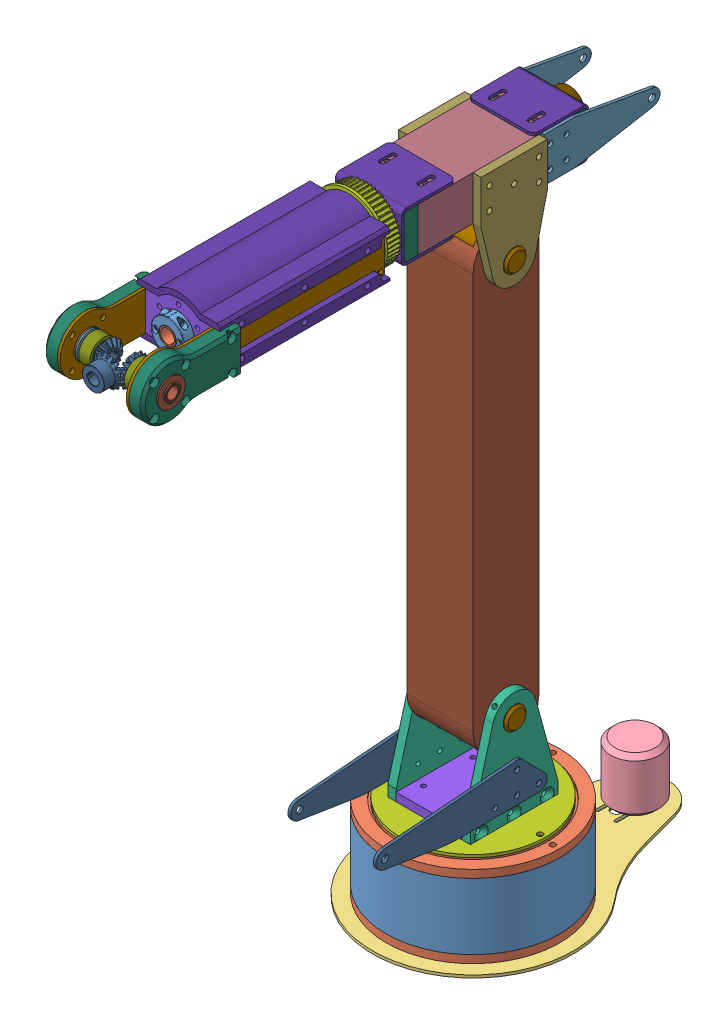
SolidWorks assembly Terry, configuration Default. Lengths in mm.
Overall size (231.75 807.08 778.1).
62 component instances, 35 part files, 0 mates.
Components (placement in the parent):
- Base-1: Base [Default] at origin size (231.75 257.05 389.29)
  - BotTurretHousing^Base-1: BotTurretHousing^Base [Default] at origin size (200 76.2 200) (virtual)
  - 8in-1: 8in [Default] at (0 42.6 0) size (200 9 200)
  - 8in-2: 8in [Default] at (0 -42.6 0) x (1 0 0) z (0 0 -1) size (200 9 200)
  - BasePlate^Base-1: BasePlate^Base [Default] at origin size (231.75 3.17 340.95) (virtual)
  - EXTENDED SHAFT KEDA 56-63 195KV Brushless Outrunner 6S 1500W v2 v2-1: EXTENDED SHAFT KEDA 56-63 195KV Brushless Outrunner 6S 1500W v2 v2 [Default] at (0 -47.1 -186.9763) x (-0.707107 0 -0.707107) z (-0.707107 0 0.707107) size (56 95.67 56)
  - BotTurretPlate^Base-1: BotTurretPlate^Base [Default] at origin size (166.96 3.17 166.96) (virtual)
  - SideTurretPlate^Base-1: SideTurretPlate^Base [Default] at origin size (9.52 224.38 101.23) (virtual)
  - SideTurretPlate^Base-2: SideTurretPlate^Base [Default] x (-1 0 0) z (0 0 -1) size (9.52 224.38 101.23) (virtual)
  - TopTurretPlate^Base-1: TopTurretPlate^Base [Default] at origin size (166.96 3.17 166.96) (virtual)
  - TopBrace^Base-1: TopBrace^Base [Default] at origin size (76.2 9.52 101.23) (virtual)
  - 6061K602_HARDENED PRECISION STEEL SHAFT-1: 6061K602_HARDENED PRECISION STEEL SHAFT [6061K602] at (0 151.875 0) size (101.6 25.4 25.4)
  - PivotPlate^Base-1: PivotPlate^Base [Default] at origin size (3.17 44.71 197.55) (virtual)
  - PivotPlate^Base-2: PivotPlate^Base [Default] at (98.425 0 0) size (3.17 44.71 197.55) (virtual)
- Shoulder-1: Shoulder [Default] at origin size (76.2 533.4 76.2)
  - Box^Shoulder-1: Box^Shoulder [Default] at origin size (76.2 533.4 76.2) (virtual)
- Forearm-1: Forearm [Default] at origin size (139.65 143.63 612.78)
  - SidePlate^Forearm-1: SidePlate^Forearm [Default] at origin size (47.62 127 76.2) (virtual)
  - SidePlate^Forearm-2: SidePlate^Forearm [Default] x (-1 0 0) z (0 0 -1) size (47.62 127 76.2) (virtual)
  - Box^Forearm-1: Box^Forearm [Default] at origin size (76.2 50.8 177.8) (virtual)
  - BackSidePlate^Forearm-1: BackSidePlate^Forearm [Default] at origin size (41.27 50.8 177.23) (virtual)
  - BackSidePlate^Forearm-2: BackSidePlate^Forearm [Default] at (79.375 0 0) size (41.27 50.8 177.23) (virtual)
  - 6061K602_HARDENED PRECISION STEEL SHAFT-1: 6061K602_HARDENED PRECISION STEEL SHAFT [6061K602] at (0 609.075 0) size (101.6 25.4 25.4)
  - BearingSpacer^Forearm-1: BearingSpacer^Forearm [Default] at origin size (76.2 50.8 22.22) (virtual)
  - 6384K367_BALL BEARING-1: 6384K367_BALL BEARING [6384K367] at (0 685.275 115.824) x (1 0 0) z (0 0 -1) size (44.45 44.45 14.3)
  - BearingHolder^Forearm-1: BearingHolder^Forearm [Default] at origin size (76.2 57.15 63.5) (virtual)
  - BearingSpacer^Forearm-2: BearingSpacer^Forearm [Default] at (0 0 25.4) x (-1 0 0) z (0 0 -1) size (76.2 50.8 22.22) (virtual)
  - BearingHolder^Forearm-2: BearingHolder^Forearm [Default] at (0 0 25.4) x (-1 0 0) z (0 0 -1) size (76.2 57.15 63.5) (virtual)
  - 6384K367_BALL BEARING-2: 6384K367_BALL BEARING [6384K367] at (0 685.275 -90.424) x (-1 0 0) z (0 0 1) size (44.45 44.45 14.3)
  - 6435K160_ONE-PIECE CLAMP-ON SHAFT COLLAR-1: 6435K160_ONE-PIECE CLAMP-ON SHAFT COLLAR [6435K16] at (0 685.275 -104.7242) x (1 0 0) z (0 0 -1) size (38.1 38.11 12.77)
  - 9677T100_CLAMP-ON SHAFT COLLAR WITH MOUNTING HOLES-1: 9677T100_CLAMP-ON SHAFT COLLAR WITH MOUNTING HOLES [9677T1] at (0 685.275 159.4517) x (0 -1 0) z (0 0 -1) size (38.14 38.1 13.27)
  - 89955K599_Tube^Forearm-1: 89955K599_Tube^Forearm [Default] at origin size (19.05 19.05 463.5) (virtual)
  - ThrustBase^Forearm-1: ThrustBase^Forearm [Default] at origin size (44.45 44.45 8.27) (virtual)
  - 5909K460_THRUST NEEDLE-ROLLER BEARING-1: 5909K460_THRUST NEEDLE-ROLLER BEARING [5909K46] at (0 685.275 131.2545) x (0 0 -1) z (1 0 0) size (0.81 31.75 31.75)
  - 5909K330_THRUST NEEDLE-ROLLER BEARING-1: 5909K330_THRUST NEEDLE-ROLLER BEARING [5909K33] at (0 685.275 132.2467) x (1 0 0) z (0 1 0) size (31.75 1.98 31.75)
  - 5909K460_THRUST NEEDLE-ROLLER BEARING-2: 5909K460_THRUST NEEDLE-ROLLER BEARING [5909K46] at (0 685.275 134.0517) x (0 0 -1) z (1 0 0) size (0.81 31.75 31.75)
  - PulleySupportPlate^Forearm-1: PulleySupportPlate^Forearm [Default] at origin size (63.5 63.5 3.17) (virtual)
  - J4Pulley-1: J4Pulley [Default] at (0 685.275 140.4017) x (-1 0 0) z (0 -1 0) size (84.06 20.68 84.06)
  - WristBase^Forearm-1: WristBase^Forearm [Default] at origin size (76.2 63.5 9.53) (virtual)
  - WristSidePlate^Forearm-1: WristSidePlate^Forearm [Default] at origin size (3.17 63.5 441.32) (virtual)
  - WristSidePlate^Forearm-2: WristSidePlate^Forearm [Default] at (79.375 0 0) size (3.17 63.5 441.32) (virtual)
  - WristBase^Forearm-2: WristBase^Forearm [Default] at (0 0 186.6233) size (76.2 63.5 9.53) (virtual)
  - 9677T100_CLAMP-ON SHAFT COLLAR WITH MOUNTING HOLES-2: 9677T100_CLAMP-ON SHAFT COLLAR WITH MOUNTING HOLES [9677T1] at (0 685.275 346.075) x (0 -1 0) z (0 0 -1) size (38.14 38.1 13.27)
  - 6843K130_MTL MITER GEAR--20 DEG PRESSURE ANGLE-1: 6843K130_MTL MITER GEAR--20 DEG PRESSURE ANGLE [6843K13] at (-31.1638 641.133 394.588) x (0 -0.999847 0.017483) z (0 0.017483 0.999847) size (34.68 21.82 34.5)
  - 6843K130_MTL MITER GEAR--20 DEG PRESSURE ANGLE-3: 6843K130_MTL MITER GEAR--20 DEG PRESSURE ANGLE [6843K13] at (-11.812 641.133 437.5638) x (0.017483 -0.999847 0) z (0.999847 0.017483 0) size (34.68 21.82 34.5)
  - 6384K361_BALL BEARING-1-1: 6384K361_BALL BEARING-1 [6384K361] at (-41.3385 685.275 406.4) x (0 0 1) z (-1 0 0) size (31.75 31.75 11.13)
  - 5909K440_THRUST NEEDLE-ROLLER BEARING-1: 5909K440_THRUST NEEDLE-ROLLER BEARING [5909K44] at (-34.5472 685.275 406.4) size (0.81 23.81 23.81)
  - 5909K310_THRUST NEEDLE-ROLLER BEARING-1: 5909K310_THRUST NEEDLE-ROLLER BEARING [5909K31] at (-32.7422 685.275 406.4) x (0 1 0) z (0 0 1) size (23.81 1.98 23.81)
  - SideMiterSpacer^Forearm-1: SideMiterSpacer^Forearm [Default] at origin size (2.03 31.75 31.75) (virtual)
  - SidePrintedSupport^Forearm-1: SidePrintedSupport^Forearm [Default] at origin size (16.21 63.5 115.89) (virtual)
  - 6384K361_BALL BEARING-1-2: 6384K361_BALL BEARING-1 [6384K361] at (-53.9115 685.275 406.4) x (0 0 1) z (1 0 0) size (31.75 31.75 11.13)
  - SidePrintedSupport^Forearm-2: SidePrintedSupport^Forearm [Default] at (0 1370.55 0) x (-1 0 0) z (0 0 1) size (16.21 63.5 115.89) (virtual)
  - 6384K361_BALL BEARING-1-3: 6384K361_BALL BEARING-1 [6384K361] at (53.9115 685.275 406.4) x (0 0 -1) z (-1 0 0) size (31.75 31.75 11.13)
  - 6384K361_BALL BEARING-1-4: 6384K361_BALL BEARING-1 [6384K361] at (41.3385 685.275 406.4) x (0 0 -1) z (1 0 0) size (31.75 31.75 11.13)
  - SideMiterSpacer^Forearm-2: SideMiterSpacer^Forearm [Default] at (0 0 812.8) x (-1 0 0) z (0 0 -1) size (2.03 31.75 31.75) (virtual)
  - 5909K440_THRUST NEEDLE-ROLLER BEARING-2: 5909K440_THRUST NEEDLE-ROLLER BEARING [5909K44] at (34.5472 685.275 406.4) x (-1 0 0) z (0 0 -1) size (0.81 23.81 23.81)
  - 5909K310_THRUST NEEDLE-ROLLER BEARING-2: 5909K310_THRUST NEEDLE-ROLLER BEARING [5909K31] at (32.7422 685.275 406.4) x (0 1 0) z (0 0 1) size (23.81 1.98 23.81)
  - 6843K130_MTL MITER GEAR--20 DEG PRESSURE ANGLE-4: 6843K130_MTL MITER GEAR--20 DEG PRESSURE ANGLE [6843K13] at (31.1638 728.9771 393.052) x (0 0.999847 -0.017483) z (0 0.017483 0.999847) size (34.68 21.82 34.5)
  - 6391K281_OIL-EMBEDDED SLEEVE BEARING-1: 6391K281_OIL-EMBEDDED SLEEVE BEARING [6391K281] at (-26.162 685.275 406.4) x (0 0 1) z (-1 0 0) size (31.78 31.78 12.7)
  - 6391K281_OIL-EMBEDDED SLEEVE BEARING-2: 6391K281_OIL-EMBEDDED SLEEVE BEARING [6391K281] at (26.162 685.275 406.4) x (0 0 1) z (-1 0 0) size (31.78 31.78 12.7)
  - WristCover^Forearm-1: WristCover^Forearm [Default] at origin size (95.25 25.4 196.15) (virtual)
  - WristCover^Forearm-2: WristCover^Forearm [Default] at (0 1370.55 0) x (-1 0 0) z (0 0 1) size (95.25 25.4 196.15) (virtual)
